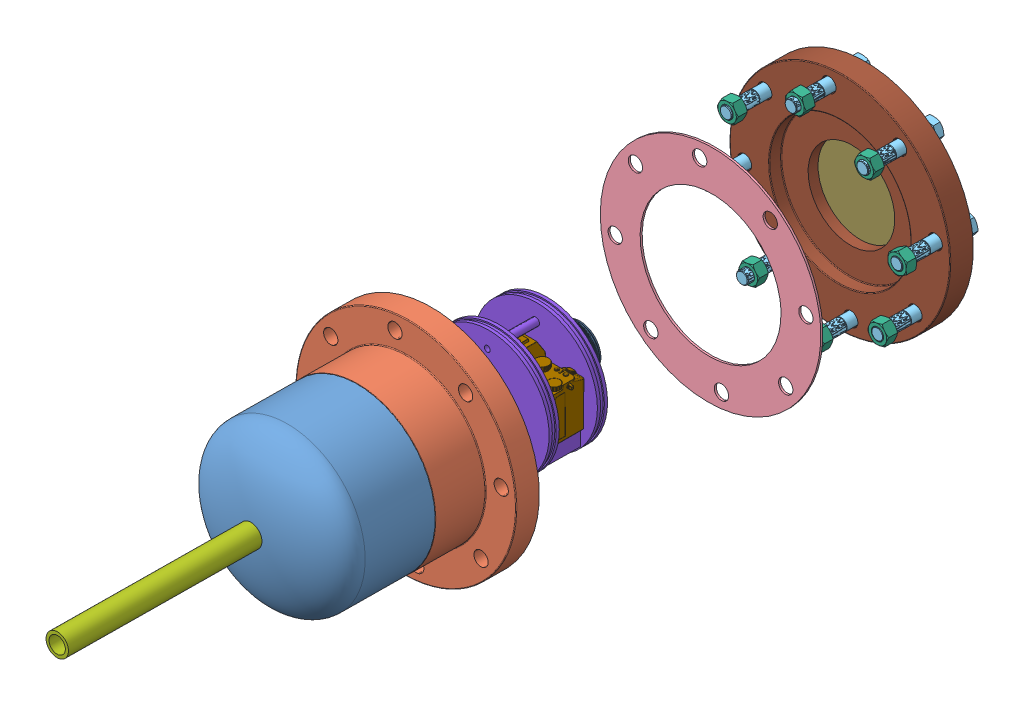
SolidWorks assembly Photogrametry_V4-PVC-apart, configuration Default. Lengths in mm.
Overall size (389.6 397.39 1323.53).
29 component instances, 13 part files, 35 mates.
Components (placement in the parent):
- 8in PVC Cap-1: 8in PVC Cap [4881K523] at (-197.711 445.5411 1109.0128) x (0.006396 0.016238 0.999848) z (-0.99998 0.000109 0.006395) size (216.92 247.14 247.14)
- 8in PVC Flange-1: 8in PVC Flange [4881K224] at (-199.5098 440.9745 827.8252) x (0.991528 0.12962 -0.008448) z (0.006396 0.016238 0.999848) size (342.9 342.9 115.89)
- 8in PVC Pipe-1: 8in PVC Pipe [48855K43] at (-198.7686 442.8563 943.695) x (0.99998 -0.000109 -0.006395) z (0.006396 0.016238 0.999848) size (219.07 219.07 203.2)
- 8in PVC Flange Closed-1: 8in PVC Flange Closed [4881K973] at (-203.8165 430.0412 154.6128) x (0.991528 0.12962 -0.008448) z (0.006396 0.016238 0.999848) size (342.9 342.9 36.51) (hidden)
- 8in Buna-N Gasket-1: 8in Buna-N Gasket [8516T54] at (-202.3564 433.748 382.8567) x (0.991528 0.12962 -0.008448) z (0.006396 0.016238 0.999848) size (342.9 342.9 3.17)
- BOLT 3-4in x 4in-1: BOLT 3-4in x 4in [92198A390] at (-55.6589 449.8836 184.1339) x (0.006396 0.016238 0.999848) z (-0.923711 -0.382898 0.012128) size (114.21 33 28.57)
- BOLT 3-4in x 4in-2: BOLT 3-4in x 4in [92198A390] at (-112.7012 548.7917 180.3993) x (0.006396 0.016238 0.999848) z (-0.923711 -0.382898 0.012128) size (114.21 33 28.57)
- BOLT 3-4in x 4in-3: BOLT 3-4in x 4in [92198A390] at (-85.3179 339.5741 184.2386) x (0.006396 0.016238 0.999848) z (-0.923711 -0.382898 0.012128) size (114.21 33 28.57)
- BOLT 3-4in x 4in-4: BOLT 3-4in x 4in [92198A390] at (-184.2691 282.5705 186.1758) x (0.006396 0.016238 0.999848) z (-0.923711 -0.382898 0.012128) size (114.21 33 28.57)
- BOLT 3-4in x 4in-5: BOLT 3-4in x 4in [92198A390] at (-321.9331 521.4781 184.7049) x (0.006396 0.016238 0.999848) z (0.4222 -0.906423 0.01202) size (114.21 33 28.57)
- BOLT 3-4in x 4in-6: BOLT 3-4in x 4in [92198A390] at (-222.9856 578.4725 182.203) x (0.006396 0.016238 0.999848) z (-0.923711 -0.382898 0.012128) size (114.21 33 28.57)
- BOLT 3-4in x 4in-9: BOLT 3-4in x 4in [92198A390] at (-351.5769 411.2074 187.2008) x (0.006396 0.016238 0.999848) z (-0.525994 0.850424 -0.010446) size (114.21 33 28.57)
- BOLT 3-4in x 4in-10: BOLT 3-4in x 4in [92198A390] at (-294.5606 312.2333 186.8661) x (0.006396 0.016238 0.999848) z (-0.923711 -0.382898 0.012128) size (114.21 33 28.57)
- NUT 3-4in-2: NUT 3-4in [92676A510] at (-54.5229 450.7088 232.3767) x (0.999988 -0.000941 -0.004773) z (0.004802 0.034121 0.999406) size (28.57 33 20.12)
- NUT 3-4in-3: NUT 3-4in [92676A510] at (-183.9607 283.3536 234.392) x (0.776919 0.629418 -0.015192) z (0.006396 0.016238 0.999848) size (28.57 33 20.12)
- NUT 3-4in-4: NUT 3-4in [92676A510] at (-294.3143 312.8586 225.3678) x (0.776919 0.629418 -0.015192) z (0.006396 0.016238 0.999848) size (28.57 33 20.12)
- NUT 3-4in-5: NUT 3-4in [92676A510] at (-85.0095 340.3571 232.4548) x (0.776919 0.629418 -0.015192) z (0.006396 0.016238 0.999848) size (28.57 33 20.12)
- NUT 3-4in-6: NUT 3-4in [92676A510] at (-351.3851 411.6941 217.1728) x (0.476506 0.879001 -0.017324) z (0.006396 0.016238 0.999848) size (28.57 33 20.12)
- NUT 3-4in-7: NUT 3-4in [92676A510] at (-321.636 522.2323 231.1455) x (-0.898727 0.438507 -0.001372) z (0.006396 0.016238 0.999848) size (28.57 33 20.12)
- NUT 3-4in-8: NUT 3-4in [92676A510] at (-222.7189 579.1494 223.8814) x (0.923711 0.382898 -0.012128) z (0.006396 0.016238 0.999848) size (28.57 33 20.12)
- NUT 3-4in-9: NUT 3-4in [92676A510] at (-112.4103 549.53 225.8644) x (0.827746 0.560918 -0.014405) z (0.006396 0.016238 0.999848) size (28.57 33 20.12)
- 5233K730_MASTERKLEER PVC TUBING-1: 5233K730_MASTERKLEER PVC TUBING [5233K73] at (-196.738 448.011 1261.0964) x (-0.006396 -0.016238 -0.999848) z (0.99998 -0.000109 -0.006395) size (304.8 34.92 34.92)
- camera case V3-1: camera case V3 [Default] at (-200.6351 438.1178 651.9256) x (-0.999819 -0.017794 0.006685) z (-0.006396 -0.016238 -0.999848) size (192 192 92)
- A7 III + FE 28-70 v4-1: A7 III + FE 28-70 v4 [Default] at (-189.5828 400.1985 680.6098) x (-0.999962 0 -0.008727) z (-0.000076 0.999962 0.008726) size (139.07 134.7 103.31)
  - A7 III + FE 28-70 v4.step-1: A7 III + FE 28-70 v4.step [Default] at origin size (139.07 134.7 103.31)
    - Sony A7 III.step-1: Sony A7 III.step [Default] at origin size (139.07 74.69 103.31)
    - Sony FE 28-70 mm f_3.5-5.6 OSS.step-1: Sony FE 28-70 mm f_3.5-5.6 OSS.step [Default] at (13.5 -93.5 40) size (72.5 83 72.5)
- 8in PVC Flange Closed - Dome Hole-1: 8in PVC Flange Closed - Dome Hole [4881K973] at (-203.8825 429.8737 144.3) x (0.991528 0.12962 -0.008448) z (0.006396 0.016238 0.999848) size (342.9 342.9 36.51)
- Custom Dome_v2.2-1: Custom Dome_v2.2 [Default] at (-203.8652 429.9175 147.0005) x (-0.924601 -0.380744 0.012098) z (0.380882 -0.924538 0.012578) size (135 55 135)
Mates (geometry in assembly coordinates):
- Coincident3: coincident anti-aligned: circle of 8in PVC Flange-1; circle of 8in PVC Pipe-1
- Concentric1: concentric anti-aligned: circle of 8in PVC Cap-1; circle of 8in PVC Pipe-1
- Concentric3: concentric anti-aligned: circle of 8in PVC Flange-1; circle of 8in Buna-N Gasket-1
- Concentric4: concentric aligned: circle of 8in PVC Flange Closed-1; circle of 8in Buna-N Gasket-1
- Concentric5: concentric aligned: circle of 8in PVC Flange Closed-1; circle of BOLT 3-4in x 4in-1
- Concentric16: concentric aligned: circle of 8in PVC Flange Closed-1; circle of BOLT 3-4in x 4in-2
- Concentric17: concentric aligned: circle of 8in PVC Flange Closed-1; circle of BOLT 3-4in x 4in-6
- Concentric18: concentric aligned: circle of 8in PVC Flange Closed-1; circle of BOLT 3-4in x 4in-5
- Concentric19: concentric aligned: circle of 8in PVC Flange Closed-1; circle of BOLT 3-4in x 4in-3
- Concentric20: concentric aligned: circle of 8in PVC Flange Closed-1; circle of BOLT 3-4in x 4in-4
- Concentric21: concentric aligned: circle of 8in PVC Flange Closed-1; circle of BOLT 3-4in x 4in-9
- Concentric22: concentric aligned: circle of 8in PVC Flange Closed-1; circle of BOLT 3-4in x 4in-10
- Concentric23: concentric aligned: circle of 8in PVC Flange Closed-1; circle of 8in Buna-N Gasket-1
- Concentric24: concentric aligned: circle of 8in PVC Flange-1; circle of 8in Buna-N Gasket-1
- Tangent2: tangent: curve of BOLT 3-4in x 4in-1; circle of NUT 3-4in-2
- Concentric26: concentric aligned: circle of BOLT 3-4in x 4in-4; circle of NUT 3-4in-3
- Concentric27: concentric aligned: circle of BOLT 3-4in x 4in-10; circle of NUT 3-4in-4
- Concentric28: concentric aligned: circle of BOLT 3-4in x 4in-3; circle of NUT 3-4in-5
- Concentric29: concentric aligned: circle of BOLT 3-4in x 4in-2; circle of NUT 3-4in-9
- Concentric30: concentric aligned: circle of BOLT 3-4in x 4in-6; circle of NUT 3-4in-8
- Concentric31: concentric aligned: circle of BOLT 3-4in x 4in-9; circle of NUT 3-4in-6
- Concentric32: concentric aligned: circle of BOLT 3-4in x 4in-5; circle of NUT 3-4in-7
- Coincident9: coincident anti-aligned: circle of 8in PVC Cap-1; circle of 5233K730_MASTERKLEER PVC TUBING-1
- Concentric33: concentric anti-aligned: circle of 8in PVC Pipe-1; circle of camera case V3-1
- Lock1: lock: unknown of camera case V3-1; unknown of A7 III + FE 28-70 v4-1/A7 III + FE 28-70 v4.step-1/Sony A7 III.step-1
- Concentric34: concentric anti-aligned: circle of 8in Buna-N Gasket-1; circle of 8in PVC Flange Closed - Dome Hole-1
- Concentric35: concentric aligned: circle of 8in Buna-N Gasket-1; circle of 8in PVC Flange Closed - Dome Hole-1
- Concentric36: concentric aligned: circle of 8in PVC Flange Closed - Dome Hole-1; circle of Custom Dome_v2.2-1
- Lock2: lock: unknown of BOLT 3-4in x 4in-5; unknown of NUT 3-4in-7
- Lock4: lock: unknown of BOLT 3-4in x 4in-2; unknown of NUT 3-4in-9
- Lock5: lock: unknown of BOLT 3-4in x 4in-1; unknown of NUT 3-4in-2
- Lock6: lock: unknown of BOLT 3-4in x 4in-3; unknown of NUT 3-4in-5
- Lock7: lock: unknown of BOLT 3-4in x 4in-4; unknown of NUT 3-4in-3
- Lock8: lock: unknown of BOLT 3-4in x 4in-10; unknown of NUT 3-4in-4
- Lock9: lock: unknown of BOLT 3-4in x 4in-6; unknown of NUT 3-4in-8
